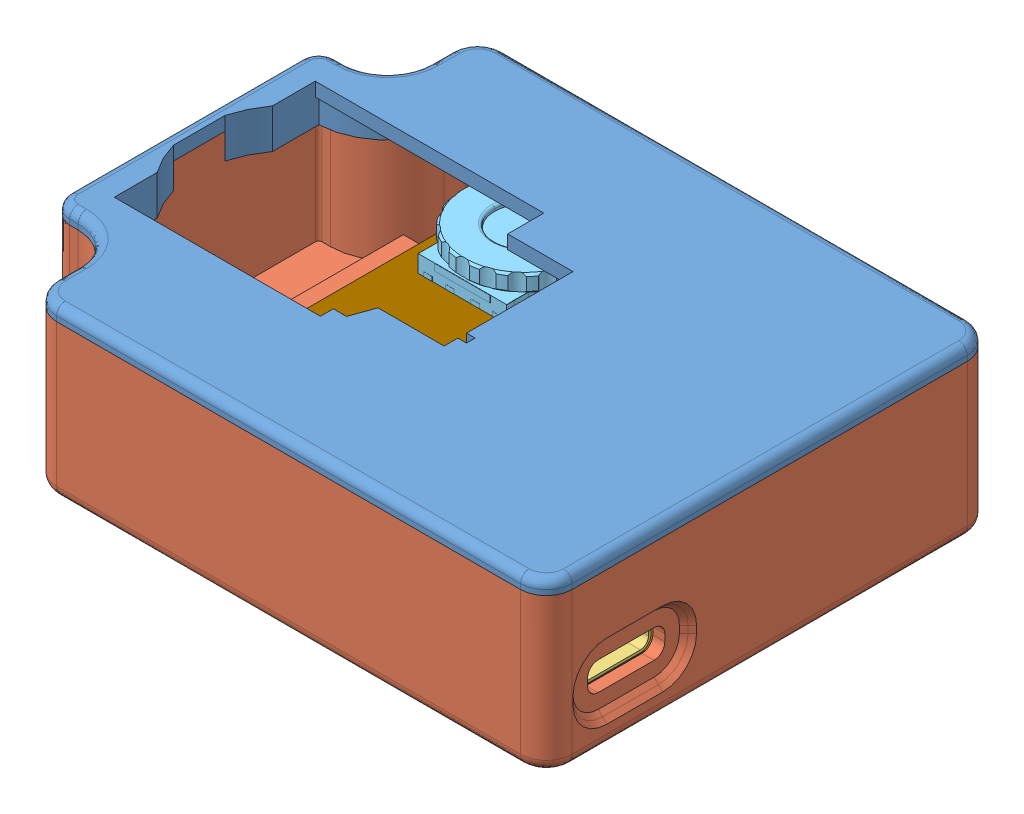
SolidWorks assembly 装配体1, configuration 默认. Lengths in mm.
Overall size (68 19.6 53.45).
32 component instances, 11 part files, 15 mates.
Components (placement in the parent):
- 零件1^装配体1-1: 零件1^装配体1 [默认] at origin size (68 4.6 52) (virtual)
- 零件2^装配体1-1: 零件2^装配体1 [默认] at origin size (68 18 52) (virtual)
- 3D_V1.1_PCB_1_2024-08-06.step-1: 3D_V1.1_PCB_1_2024-08-06.step [默认] at (19.1386 -14.6 60.9302) x (-1 0 0) z (0 1 0) size (54.22 49.65 5.6)
  - oSxv-USB1.step-1: oSxv-USB1.step [默认] at (-5.08 -35.5601 1.6) x (0 -1 0) z (0 0 1) size (8.94 7.58 4.16)
    - USB-C-SMD_TYPE-C-6PIN-2MD-073.step-1: USB-C-SMD_TYPE-C-6PIN-2MD-073.step [默认] at origin size (8.94 7.58 4.16)
      - COMPOUND.step-1: COMPOUND.step [默认] at origin size (8.94 7.58 4.16)
  - oSxv-ANT1.step-1: oSxv-ANT1.step [默认] at (-5.08 -69.0881 1.6) size (3 3.12 1.26)
    - ANT-SMD_KH-IPEX-K501-29.step-1: ANT-SMD_KH-IPEX-K501-29.step [默认] at origin size (3 3.12 1.26)
      - SOLID.step-1: SOLID.step [默认] at origin size (3 3.12 1.26)
  - oSxv-U6.step-1: oSxv-U6.step [默认] at (36.0681 -68.8341 1.6) x (-1 0 0) z (0 0 1) size (14.5 14.57 4.5)
    - SW-SMD_SIQ-02FVS3_1.step-1: SW-SMD_SIQ-02FVS3_1.step [默认] at origin size (14.5 14.57 4.5)
      - COMPOUND-0.step-1: COMPOUND-0.step [默认] at origin size (14.5 14.57 4.5)
  - oSxv-SW2.step-1: oSxv-SW2.step [默认] at (10.033 -73.1521 1.6) x (-1 0 0) z (0 0 1) size (7.8 3.7 4.25)
    - KEY-SMD_4P-L7.8-W2.8-P4.20-EH.step-1: KEY-SMD_4P-L7.8-W2.8-P4.20-EH.step [默认] at origin size (7.8 3.7 4.25)
      - COMPOUND-1.step-1: COMPOUND-1.step [默认] at origin size (7.8 3.7 4.25)
  - oSxv-SW3.step-1: oSxv-SW3.step [默认] at (19.812 -73.1521 1.6) x (-1 0 0) z (0 0 1) size (7.8 3.7 4.25)
    - KEY-SMD_4P-L7.8-W2.8-P4.20-EH.step-1: KEY-SMD_4P-L7.8-W2.8-P4.20-EH.step [默认] at origin size (7.8 3.7 4.25)
      - COMPOUND-1.step-1: COMPOUND-1.step [默认] at origin size (7.8 3.7 4.25)
  - oSxv-SW1.step-1: oSxv-SW1.step [默认] at (-3.937 -73.1521 1.6) x (-1 0 0) z (0 0 1) size (7.8 3.7 4.25)
    - KEY-SMD_4P-L7.8-W2.8-P4.20-EH.step-1: KEY-SMD_4P-L7.8-W2.8-P4.20-EH.step [默认] at origin size (7.8 3.7 4.25)
      - COMPOUND-1.step-1: COMPOUND-1.step [默认] at origin size (7.8 3.7 4.25)
  - oSxv-U1.step-1: oSxv-U1.step [默认] at (26.0351 -43.6881 1.6) size (16 16 1.5)
    - LQFP-128_L14.0-W14.0-P0.40-LS16.0-BL-EP5.6.step-1: LQFP-128_L14.0-W14.0-P0.40-LS16.0-BL-EP5.6.step [默认] at origin size (16 16 1.5)
      - SOLID-2.step-1: SOLID-2.step [默认] at origin size (16 16 1.5)
  - oSxv-FPC2.step-1: oSxv-FPC2.step [默认] at (40.5131 -36.3221 1.6) x (0 1 0) z (0 0 1) size (13.2 3.55 1.02)
    - FFC-SMD_F0302-B-39-10G-R.step-1: FFC-SMD_F0302-B-39-10G-R.step [默认] at origin size (13.2 3.55 1.02)
      - COMPOUND-3.step-1: COMPOUND-3.step [默认] at origin size (13.2 3.55 1.02)
  - Board.step-1: Board.step [默认] at origin size (54.17 46.07 1.6)
- 屏幕模型^装配体1-1: 屏幕模型^装配体1 [默认] at (15.105 -16.8 -0.6836) size (54.2 2.2 46) (virtual)
- 按钮^装配体1-1: 按钮^装配体1 [默认] at (28.2514 -12.2267 -14.7656) x (1 0 0) z (0 1 0) size (4.8 2.8 7.8) (virtual)
- 按钮^装配体1-2: 按钮^装配体1 [默认] at (4.5514 -12.2267 -14.7656) x (1 0 0) z (0 1 0) size (4.8 2.8 7.8) (virtual)
- 按钮^装配体1-3: 按钮^装配体1 [默认] at (14.2514 -12.2267 -14.7656) x (1 0 0) z (0 1 0) size (4.8 2.8 7.8) (virtual)
Mates (geometry in assembly coordinates):
- 距离3: distance = 0.2 mm anti-aligned: plane of 零件2^装配体1-1 through (29.3589 -89.5881 -14.3656) normal (-1 0 0); plane of 3D_V1.1_PCB_1_2024-08-06.step-1/Board.step-1 through (29.1589 -14.6 -13.003) normal (1 0 0)
- 距离1: distance = 0.1 mm anti-aligned: plane of 零件2^装配体1-1 through (-25.2411 -89.5881 31.9344) normal (0 0 -1); plane of 3D_V1.1_PCB_1_2024-08-06.step-1/Board.step-1 through (27.9216 -14.6 31.8344) normal (0 0 1)
- 距离2: distance = 2.2 mm anti-aligned: plane of 零件2^装配体1-1 through (28.7589 -16.8 -13.3656) normal (0 1 0); plane of 3D_V1.1_PCB_1_2024-08-06.step-1/Board.step-1 through (2.0715 -14.6 8.7971) normal (0 -1 0)
- 重合7: coincident anti-aligned: plane of 零件2^装配体1-1 through (28.7589 -16.8 -13.3656) normal (0 1 0); plane of 屏幕模型^装配体1-1 through (15.105 -16.8 -0.6836) normal (0 -1 0)
- 重合8: coincident anti-aligned: plane of 零件2^装配体1-1 through (-25.2411 -89.5881 -14.3656) normal (0 0 1); plane of 屏幕模型^装配体1-1 through (-24.8411 -14.6 -14.3656) normal (0 0 -1)
- 重合9: coincident anti-aligned: plane of 零件2^装配体1-1 through (29.3589 -89.5881 -14.3656) normal (-1 0 0); plane of 屏幕模型^装配体1-1 through (29.3589 -14.6 -14.3656) normal (1 0 0)
- 距离4: distance = 0.1 mm anti-aligned: plane of 零件2^装配体1-1 through (25.5589 -12.8 35.6354) normal (0 1 0); plane of 按钮^装配体1-1 through (28.2514 -12.7 -17.5656) normal (0 -1 0)
- 距离5: distance = 0.1 mm anti-aligned: plane of 零件2^装配体1-1 through (25.5589 -9.8 35.6354) normal (-1 0 0); plane of 按钮^装配体1-1 through (25.4589 -12.2267 -15.5656) normal (1 0 0)
- 重合13: coincident anti-aligned: plane of 零件2^装配体1-1 through (0 0 -15.5656) normal (0 0 1); plane of 按钮^装配体1-1 through (28.2514 -12.2267 -15.5656) normal (0 0 -1)
- 距离6: distance = 0.1 mm anti-aligned: plane of 按钮^装配体1-3 through (11.4589 -12.2267 -15.5656) normal (1 0 0); plane of 零件2^装配体1-1 through (11.5589 -9.8 35.6354) normal (-1 0 0)
- 距离7: distance = 0.1 mm anti-aligned: plane of 按钮^装配体1-3 through (14.2514 -9.9 -17.5656) normal (0 1 0); plane of 零件2^装配体1-1 through (11.5589 -9.8 35.6354) normal (0 -1 0)
- 重合16: coincident anti-aligned: plane of 零件2^装配体1-1 through (0 0 -15.5656) normal (0 0 1); plane of 按钮^装配体1-3 through (14.2514 -12.2267 -15.5656) normal (0 0 -1)
- 距离8: distance = 0.1 mm anti-aligned: plane of 按钮^装配体1-2 through (1.7589 -12.2267 -15.5656) normal (1 0 0); plane of 零件2^装配体1-1 through (1.8589 -9.8 35.6354) normal (-1 0 0)
- 距离9: distance = 0.1 mm anti-aligned: plane of 按钮^装配体1-2 through (4.5514 -9.9 -17.5656) normal (0 1 0); plane of 零件2^装配体1-1 through (1.8589 -9.8 35.6354) normal (0 -1 0)
- 重合19: coincident anti-aligned: plane of 零件2^装配体1-1 through (0 0 -15.5656) normal (0 0 1); plane of 按钮^装配体1-2 through (4.5514 -12.2267 -15.5656) normal (0 0 -1)
